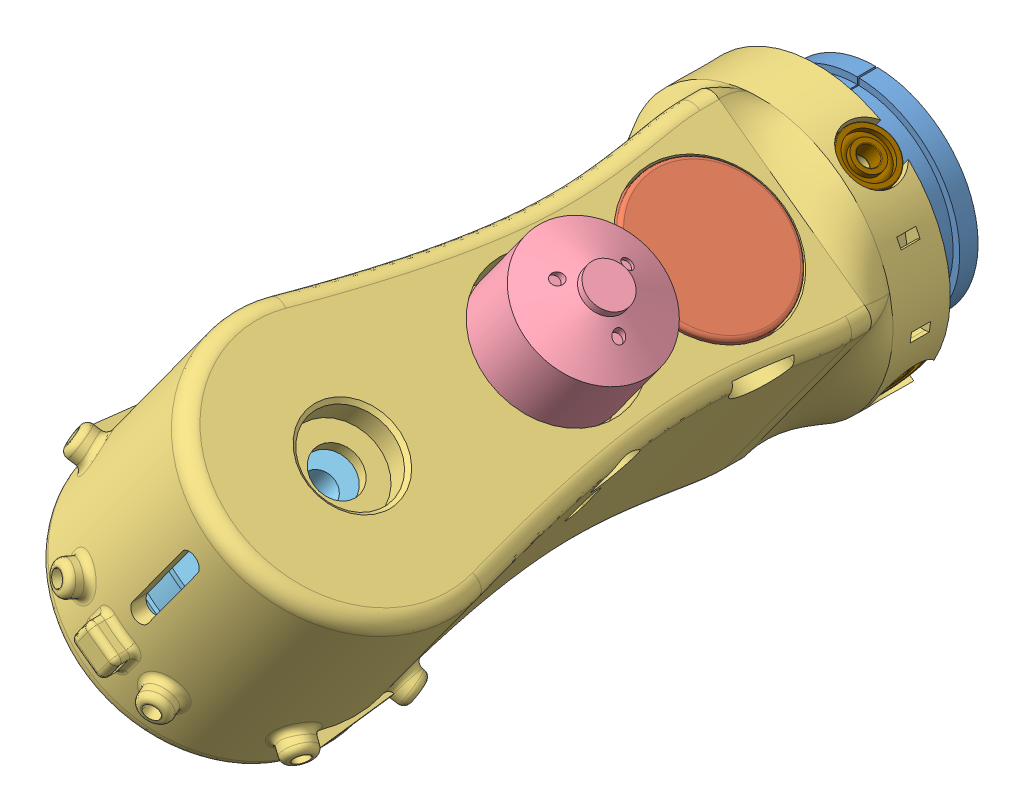
SolidWorks assembly A5 Assembly, configuration Default. Lengths in mm.
Overall size (117.85 116.54 195.47).
16 component instances, 13 part files, 42 mates.
Components (placement in the parent):
- A5D1 - Input Ring-3: A5D1 - Input Ring [Default] at (-5.5765 -43.1726 42.7362) size (53.6 53.6 26.97)
- Encoder600PR-2: Encoder600PR [Default] at (-32.2392 -16.8999 55.5428) x (0.809017 -0.587785 -0.000664) z (-0.000537 0.000391 -1) size (38 53 38)
- A5D2 - Main-2: A5D2 - Main [Default] at (-51.3422 -43.193 34.1028) x (0.587785 0.809017 0) z (0.809017 -0.587785 0) size (80.94 180.44 86.87)
- Propdrive v2 3536-910kv-2: Propdrive v2 3536-910kv [Default] at (-19.21 1.0333 95.5428) x (0.576802 -0.419071 -0.701198) z (-0.567281 0.412154 -0.712967) size (35.77 56 35.77)
- Pulley HTD_3mm T60 D8-1: Pulley HTD_3mm T60 D8 [Default] at (-56.0759 -49.7083 149.1028) x (-0.142543 0.103564 -0.984356) z (0.79636 -0.57859 -0.176193) size (60 25 60)
- radial ball bearing_68_am-1: radial ball bearing_68_am [AFBMA 20.1 - 17-50 - 40,DE,NC,40_68] at (-68.0941 -66.25 149.1028) x (0.587785 0.809017 0) z (-0.798405 0.580075 -0.161441) size (6 62 62) (hidden)
- A5D7 - Encoder Sun-1: A5D7 - Encoder Sun [Default] at (-53.2293 -54.7697 50.8784) x (0.72854 -0.529315 0.434804) z (-0.587785 -0.809017 0) size (17 16.93 18)
- A5D3 - Output Ring-1: A5D3 - Output Ring [Default] at (-64.8511 -62.4299 149.1136) x (0.809017 -0.587785 0) z (0.587785 0.809017 0) size (60.74 61.32 16.45)
- radial ball bearing_68_din-1: radial ball bearing_68_din [DIN 625 - 608 - 8,DE,NC,8_68] at (-71.9147 -71.5086 95.5428) x (-0.587785 -0.809017 0) z (0.370529 -0.269205 0.888953) size (7 22 22)
- radial ball bearing_68_iso-1: radial ball bearing_68_iso [ISO 15 RBB - 105 - 8,SI,NC,8_68] at (-69.5636 -68.2725 15.1028) x (-0.587785 -0.809017 0) z (-0.658083 0.478125 0.581656) size (5 14 14)
- radial ball bearing_68_iso-2: radial ball bearing_68_iso [ISO 15 RBB - 105 - 8,SI,NC,8_68] at (-26.2627 -61.4143 15.1028) x (0.809017 -0.587785 0) z (-0.478125 -0.658083 0.581656) size (5 14 14)
- radial ball bearing_68_iso-3: radial ball bearing_68_iso [ISO 15 RBB - 105 - 8,SI,NC,8_68] at (-33.1209 -18.1135 15.1028) x (0.587785 0.809017 0) z (0.658083 -0.478125 0.581656) size (5 14 14)
- radial ball bearing_68_iso-4: radial ball bearing_68_iso [ISO 15 RBB - 105 - 8,SI,NC,8_68] at (-76.4218 -24.9717 15.1028) x (-0.809017 0.587785 0) z (0.478125 0.658083 0.581656) size (5 14 14)
- A5D5 - BLDC Sun-1: A5D5 - BLDC Sun [Default] at (-43.3092 -32.1364 95.5428) x (0.221765 -0.161121 -0.961697) z (-0.587785 -0.809017 0) size (24 24 50.67)
- A5D6 - Axis holder-2: A5D6 - Axis holder [Default] at (-67.5063 -65.441 95.5428) x (-0.572061 0.415627 -0.707107) z (-0.572061 0.415627 0.707107) size (49 11 49)
- Bearing - I50 - O62 - D6-1: Bearing - I50 - O62 - D6 [AFBMA 20.1 - 17-50 - 40,DE,NC,40_68] at (-68.0961 -66.2527 149.1028) x (0.587785 0.809017 0) z (-0.219405 0.159407 0.962523) size (6 62 62)
Mates (geometry in assembly coordinates):
- Concentric1: concentric anti-aligned: cylinder of A5D1 - Input Ring-3 through (-51.3422 -43.193 -79.1326) axis (0 0 1) radius 25.06; cylinder of ? through (-51.3422 -43.193 29.1028) axis (0 0 -1) radius 35
- Concentric2: concentric anti-aligned: cylinder of A5D1 - Input Ring-3 through (-30.7664 -14.8734 15.1028) axis (-0.587785 -0.809017 0) radius 2.55; cylinder of ? through (-71.9153 -71.5094 15.1028) axis (0.587785 0.809017 0) radius 2.65
- Parallel1: parallel: plane of ? through (-1.7276 -17.4368 149.1028) normal (0 0 1); plane of ? through (-68.9852 -51.0139 66.147) normal (0 0 1)
- Concentric5: concentric anti-aligned: cylinder of A5D1 - Input Ring-3 through (-51.3422 -43.193 -79.1326) axis (0 0 1) radius 25.06; circle of ?
- Concentric8: concentric: cylinder of ? through (-93.1535 -8.4767 131.0901) axis (0.991377 -0.131042 0) radius 21.5; cylinder of ? through (-73.1457 -29.2361 120.6552) axis (-0.991377 0.131042 0) radius 6.975
- Distance4: distance = 5 mm: plane of ? through (-72.8157 -26.622 111.8312) normal (0.991377 -0.131042 0); plane of ? through (-64.5349 -2.1308 145.6552) normal (0.991377 -0.131042 0)
- Parallel2: parallel: plane of ? through (-36.806 -41.1325 79.9056) normal (0.991948 0.126646 0); plane of A5D2 - Main-2 through (-63.4937 -0.3725 184.1028) normal (-0.587785 -0.809017 0)
- Parallel3: parallel anti-aligned: plane of A5D2 - Main-2 through (-61.1426 2.8635 184.1028) normal (0.587785 0.809017 0); plane of ? through (-82.4856 -46.4154 79.1646) normal (-0.939424 -0.342757 0)
- Concentric9: concentric aligned: cylinder of A5D3-2 through (-71.9205 -71.5165 149.1028) axis (0.587785 0.809017 0) radius 30.95; cylinder of Pulley HTD_3mm T60 D8-1 through (-55.1942 -48.4947 149.1028) axis (0.587785 0.809017 0) radius 28.9532
- Concentric10: concentric aligned: cylinder of A5D2 - Main-2 through (-71.9205 -71.5165 149.1028) axis (0.587785 0.809017 0) radius 30.95; cylinder of A5D3 - Output Ring-1 through (-116.6118 -133.0288 149.1028) axis (0.587785 0.809017 0) radius 30.95
- Concentric11: concentric aligned: cylinder of A5D3-2 through (-71.9205 -71.5165 149.1028) axis (0.587785 0.809017 0) radius 30.95; cylinder of radial ball bearing_68_am-1 through (-80.2245 -82.9461 149.1028) axis (0.587785 0.809017 0) radius 31
- Concentric14: concentric aligned: cylinder of A5D2 - Main-2 through (-102.1105 -26.1507 25.7617) axis (0.309597 -0.224936 0.92388) radius 2.05; cylinder of A5D3 - Output Ring-1 through (-53.3633 -61.5676 171.2297) axis (0.309597 -0.224936 0.92388) radius 2.1
- Concentric15: concentric aligned: cylinder of A5D1 Ring From A4-3 through (-51.3422 -43.193 -79.1326) axis (0 0 1) radius 25.06; cylinder of A5D3-2 through (-51.3422 -43.193 9.1028) axis (0 0 1) radius 35
- Concentric16: concentric anti-aligned: cylinder of A5D1 Ring From A4-3 through (-71.9181 -71.5126 15.1028) axis (0.587785 0.809017 0) radius 2.55; cylinder of A5D3-2 through (-27.555 -10.4527 15.1028) axis (-0.587785 -0.809017 0) radius 2.55
- Parallel9: parallel aligned: plane of Encoder600PR-2 through (-52.8117 -45.2155 55.5428) normal (-0.587785 -0.809017 0); plane of A5D3-2 through (-98.1731 -48.1045 184.1028) normal (-0.587785 -0.809017 0)
- Parallel10: parallel aligned: plane of A5D3-2 through (-98.1731 -48.1045 184.1028) normal (-0.587785 -0.809017 0); plane of Propdrive v2 3536-910kv-2 through (-40.958 -28.9004 95.5428) normal (-0.587785 -0.809017 0)
- Distance8: distance = 1 mm: plane of A5D3 - Output Ring-1 through (-56.3576 -50.7396 149.1136) normal (0.587785 0.809017 0); plane of Pulley HTD_3mm T60 D8-1 through (-56.0759 -49.7083 149.1028) normal (-0.587785 -0.809017 0)
- Coincident15: coincident aligned: plane of Pulley HTD_3mm T60 D8-1 through (-56.0759 -49.7083 149.1028) normal (-0.587785 -0.809017 0); plane of ? through (-56.2404 -49.9348 95.5428) normal (-0.587785 -0.809017 0)
- Coincident13: coincident: plane of A5D3-2 through (-51.3422 -43.193 34.1028) normal (0.809017 -0.587785 0); line of Propdrive v2 3536-910kv-2 through (-52.126 -44.2717 95.5428) axis (0.587785 0.809017 0)
- Distance9: distance = 53.56 mm: cylinder of Pulley HTD_3mm T60 D8-1 through (-47.8469 -38.382 149.1028) axis (-0.587785 -0.809017 0) radius 4; cylinder of Propdrive v2 3536-910kv-2 through (-20.3856 -0.5848 95.5428) axis (0.587785 0.809017 0) radius 5.5
- Concentric25: concentric aligned: cylinder of Propdrive v2 3536-910kv-2 through (-52.126 -44.2717 95.5428) axis (0.587785 0.809017 0) radius 2.5; cylinder of ? through (-56.2404 -49.9348 95.5428) axis (0.587785 0.809017 0) radius 2.5
- Concentric27: concentric: cylinder of ? through (-38.7049 -25.7991 95.5428) axis (-0.587785 -0.809017 0) radius 7; cylinder of ? through (-40.96 -28.903 95.5428) axis (0.587785 0.809017 0) radius 8.75
- Coincident16: coincident anti-aligned: plane of Propdrive v2 3536-910kv-2 through (-40.958 -28.9004 95.5428) normal (-0.587785 -0.809017 0); plane of ? through (-38.6088 -25.667 95.5428) normal (0.587785 0.809017 0)
- Concentric28: concentric anti-aligned: cylinder of Propdrive v2 3536-910kv-2 through (-30.9281 -30.0072 104.4549) axis (-0.587785 -0.809017 0) radius 1.5; cylinder of ? through (-33.2212 -34.5256 103.5895) axis (0.587785 0.809017 0) radius 1.6
- Coincident17: coincident anti-aligned: plane of Encoder600PR-2 through (-52.8117 -45.2155 55.5428) normal (-0.587785 -0.809017 0); plane of A5D3-2 through (-52.8117 -45.2155 55.5428) normal (0.587785 0.809017 0)
- Concentric29: concentric aligned: cylinder of Encoder600PR-2 through (-52.8117 -45.2155 55.5428) axis (0.587785 0.809017 0) radius 19; cylinder of A5D3-2 through (-75.1295 -75.9333 55.5428) axis (0.587785 0.809017 0) radius 19.5
- Coincident18: coincident anti-aligned: plane of A5D3-2 through (-40.958 -28.9004 95.5428) normal (0.587785 0.809017 0); plane of Propdrive v2 3536-910kv-2 through (-40.958 -28.9004 95.5428) normal (-0.587785 -0.809017 0)
- Concentric34: concentric aligned: cylinder of Encoder600PR-2 through (-63.3918 -59.7778 55.5428) axis (0.587785 0.809017 0) radius 3; cylinder of A5D8-1 through (-63.0979 -59.3733 55.5428) axis (0.587785 0.809017 0) radius 3.1
- Coincident22: coincident anti-aligned: plane of Encoder600PR-2 through (-60.5186 -50.7408 74.5448) normal (-0.587785 -0.809017 0); plane of A5D8-1 through (-53.8318 -55.599 50.8784) normal (0.587785 0.809017 0)
- Concentric35: concentric aligned: cylinder of A5D3-2 through (-71.9205 -71.5165 149.1028) axis (0.587785 0.809017 0) radius 30.95; cylinder of A5D4 Ring To A6_50version-1 through (-116.6118 -133.0288 149.1028) axis (0.587785 0.809017 0) radius 30.95
- Concentric36: concentric anti-aligned: cylinder of A5D3-2 through (4.8901 -103.8912 115.4809) axis (-0.747434 0.543043 0.382683) radius 2.05; cylinder of A5D4 Ring To A6_50version-1 through (-42.8771 -69.1863 139.9376) axis (0.747434 -0.543043 -0.382683) radius 2.1
- Concentric38: concentric aligned: cylinder of A5D3-2 through (-67.8002 -65.8455 15.1028) axis (-0.587785 -0.809017 0) radius 7.5; cylinder of radial ball bearing_68_iso-1 through (-57.4332 -51.5764 15.1028) axis (-0.587785 -0.809017 0) radius 7
- Coincident24: coincident anti-aligned: plane of A5D3-2 through (-68.0941 -66.25 34.1028) normal (-0.587785 -0.809017 0); plane of radial ball bearing_68_iso-1 through (-66.2824 -67.5662 18.2346) normal (0.587785 0.809017 0)
- Concentric39: concentric aligned: cylinder of Propdrive v2 3536-910kv-2 through (-52.126 -44.2717 95.5428) axis (0.587785 0.809017 0) radius 2.5; cylinder of A5D5 - BLDC Sun-1 through (-55.9466 -49.5303 95.5428) axis (0.587785 0.809017 0) radius 2.55
- Concentric40: concentric anti-aligned: cylinder of A5D2 - Main-2 through (-27.555 -10.4527 95.5428) axis (-0.587785 -0.809017 0) radius 12.5; cylinder of A5D6-2 through (-69.8575 -68.677 95.5428) axis (0.587785 0.809017 0) radius 12.45
- Coincident26: coincident anti-aligned: plane of A5D2 - Main-2 through (-98.1731 -48.1045 184.1028) normal (-0.587785 -0.809017 0); plane of A5D6-2 through (-69.8575 -68.677 95.5428) normal (0.587785 0.809017 0)
- Concentric41: concentric anti-aligned: cylinder of A5D2 - Main-2 through (-16.1138 -18.7652 109.685) axis (-0.587785 -0.809017 0) radius 1.5; cylinder of A5D6-2 through (-60.4735 -79.8211 109.685) axis (0.587785 0.809017 0) radius 1.55
- Concentric42: concentric anti-aligned: cylinder of radial ball bearing_68_din-1 through (-59.7843 -54.8125 95.5428) axis (-0.587785 -0.809017 0) radius 11; cylinder of A5D6-2 through (-73.972 -74.3401 95.5428) axis (0.587785 0.809017 0) radius 11
- Coincident27: coincident anti-aligned: plane of radial ball bearing_68_din-1 through (-63.4568 -73.3274 91.4666) normal (0.587785 0.809017 0); plane of A5D6-2 through (-69.8575 -68.677 95.5428) normal (-0.587785 -0.809017 0)
- Coincident28: coincident anti-aligned: plane of A5D2 - Main-2 through (-43.3092 -32.1364 95.5428) normal (-0.587785 -0.809017 0); plane of A5D5 - BLDC Sun-1 through (-43.3092 -32.1364 95.5428) normal (0.587785 0.809017 0)
- Concentric43: concentric: cylinder of A5D2 - Main-2 through (-71.9205 -71.5165 149.1028) axis (0.587785 0.809017 0) radius 30.95; cylinder of Bearing - I50 - O62 - D6-1 through (-80.2265 -82.9488 149.1028) axis (0.587785 0.809017 0) radius 31
- Coincident29: coincident anti-aligned: plane of A5D3 - Output Ring-1 through (-66.3327 -63.8256 149.1028) normal (-0.587785 -0.809017 0); plane of Bearing - I50 - O62 - D6-1 through (-90.2387 -46.4569 140.777) normal (0.587785 0.809017 0)
